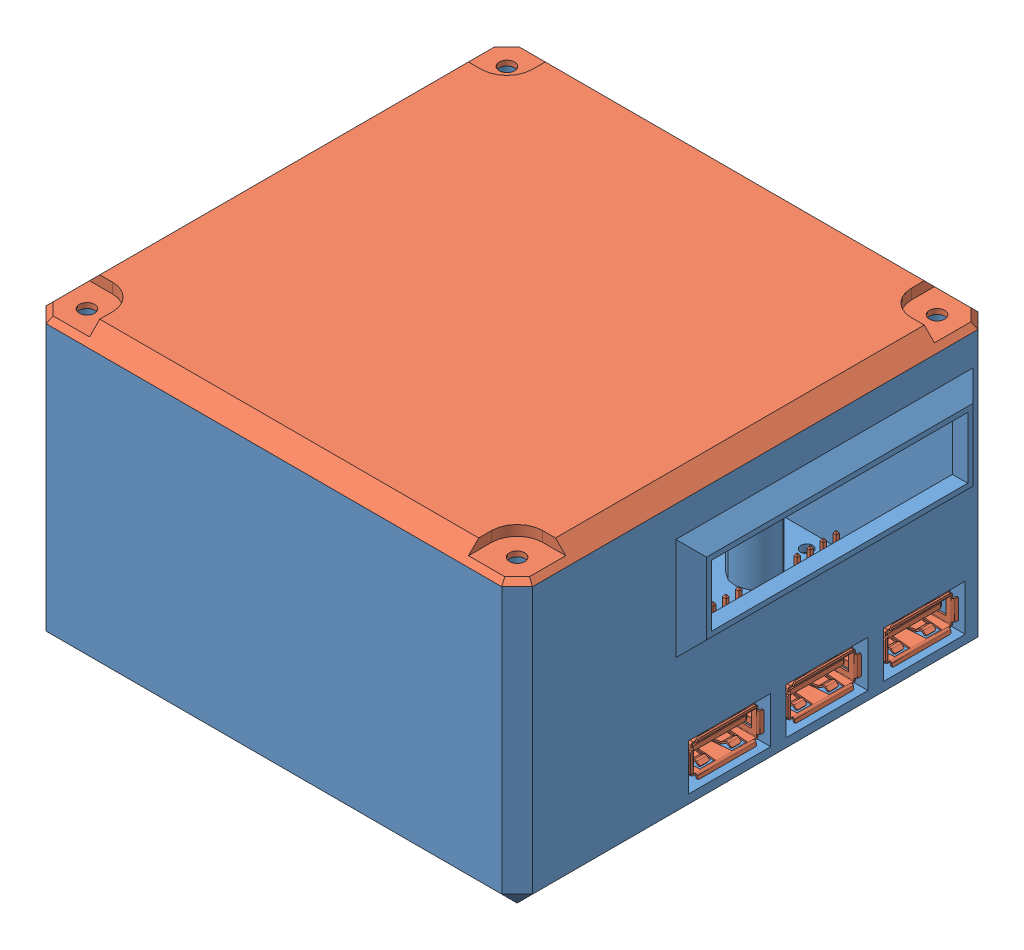
SolidWorks assembly NEW Arduino Case Assembly, configuration Default. Lengths in mm.
Overall size (98 58 93).
56 component instances, 22 part files, 33 mates.
Components (placement in the parent):
- NEW Mega 2560 Pro embed Case-1: NEW Mega 2560 Pro embed Case [Default] at origin size (98 55 93)
- NEW Mega 2560 Pro embed Case LID-1: NEW Mega 2560 Pro embed Case LID [Default] at (0 56 0) size (95 3 93)
- MEGA 2560 PRO (EMBED)-1: MEGA 2560 PRO (EMBED) [Default] at (-24.5 4 -15.5) x (1 0 0) z (0 1 0) size (38 54.09 6.02)
  - MEGA 2560 PRO (EMBED)(2)^MEGA 2560 PRO (EMBED)-1: MEGA 2560 PRO (EMBED)(2)^MEGA 2560 PRO (EMBED) [Default] at origin size (38 54.09 6.02) (virtual)
    - Mega 2560 Pro - Board^MEGA 2560 PRO (EMBED)(2)_MEGA 2560 PRO (EMBED)-1: Mega 2560 Pro - Board^MEGA 2560 PRO (EMBED)(2)_MEGA 2560 PRO (EMBED) [Default] at origin size (38 54 1.78) (virtual)
    - SOT223-3^MEGA 2560 PRO (EMBED)(2)_MEGA 2560 PRO (EMBED)-1: SOT223-3^MEGA 2560 PRO (EMBED)(2)_MEGA 2560 PRO (EMBED) [Default] at (-7.7036 13.3224 1.6256) x (-1 0 0) z (0 0 1) size (6.5 7.07 1.6) (virtual)
    - SOT223-3^MEGA 2560 PRO (EMBED)(2)_MEGA 2560 PRO (EMBED)-2: SOT223-3^MEGA 2560 PRO (EMBED)(2)_MEGA 2560 PRO (EMBED) [Default] at (-7.5781 23.9617 1.6256) x (-1 0 0) z (0 0 1) size (6.5 7.07 1.6) (virtual)
    - ATmega2560-16AU^MEGA 2560 PRO (EMBED)(2)_MEGA 2560 PRO (EMBED)-1: ATmega2560-16AU^MEGA 2560 PRO (EMBED)(2)_MEGA 2560 PRO (EMBED) [Default] at (0.2253 -9.3836 1.5256) x (0.707107 -0.707107 0) z (0 0 1) size (16 16 1.21) (virtual)
    - SOIC -16^MEGA 2560 PRO (EMBED)(2)_MEGA 2560 PRO (EMBED)-1: SOIC -16^MEGA 2560 PRO (EMBED)(2)_MEGA 2560 PRO (EMBED) [Default] at (0.546 8.9647 1.4756) x (0 1 0) z (1 0 0) size (6 1.4 9.9) (virtual)
    - Crystal Oscillator (SMD)^MEGA 2560 PRO (EMBED)(2)_MEGA 2560 PRO (EMBED)-1: Crystal Oscillator (SMD)^MEGA 2560 PRO (EMBED)(2)_MEGA 2560 PRO (EMBED) [Default] at (-10.7852 -19.6364 2.54) x (0 -1 0) z (0 0 1) size (13.06 4.55 4.32) (virtual)
    - Crystal Oscillator (SMD)^MEGA 2560 PRO (EMBED)(2)_MEGA 2560 PRO (EMBED)-2: Crystal Oscillator (SMD)^MEGA 2560 PRO (EMBED)(2)_MEGA 2560 PRO (EMBED) [Default] at (10.6809 3.6875 2.54) x (0 -1 0) z (0 0 1) size (13.06 4.55 4.32) (virtual)
    - 1206 Capacitor^MEGA 2560 PRO (EMBED)(2)_MEGA 2560 PRO (EMBED)-1: 1206 Capacitor^MEGA 2560 PRO (EMBED)(2)_MEGA 2560 PRO (EMBED) [Default] at (-3.8106 17.9279 1.6231) x (0 -1 0) z (0 0 1) size (3.2 1.6 1.6) (virtual)
    - Fuse (1206) - Green^MEGA 2560 PRO (EMBED)(2)_MEGA 2560 PRO (EMBED)-1: Fuse (1206) - Green^MEGA 2560 PRO (EMBED)(2)_MEGA 2560 PRO (EMBED) [Default] at (-0.2207 16.3875 1.6281) x (0 -1 0) z (0 0 1) size (3.28 1.75 0.87) (virtual)
    - Diode - SMD - DO-214AC^MEGA 2560 PRO (EMBED)(2)_MEGA 2560 PRO (EMBED)-1: Diode - SMD - DO-214AC^MEGA 2560 PRO (EMBED)(2)_MEGA 2560 PRO (EMBED) [Default] at (-1.7706 25.543 1.4756) x (0 -1 0) z (0 0 1) size (5.6 2.95 2.91) (virtual)
    - USB - Micro^MEGA 2560 PRO (EMBED)(2)_MEGA 2560 PRO (EMBED)-1: USB - Micro^MEGA 2560 PRO (EMBED)(2)_MEGA 2560 PRO (EMBED) [Default] at (2.2104 21.1734 1.3475) x (-1 0 0) z (0 1 0) size (7.92 3.01 5.67) (virtual)
    - 0603 Capacitor^MEGA 2560 PRO (EMBED)(2)_MEGA 2560 PRO (EMBED)-1: 0603 Capacitor^MEGA 2560 PRO (EMBED)(2)_MEGA 2560 PRO (EMBED) [Default] at (10.7145 18.9901 1.6231) x (0 -1 0) z (0 0 1) size (1.6 0.84 0.84) (virtual)
    - 0603 Capacitor^MEGA 2560 PRO (EMBED)(2)_MEGA 2560 PRO (EMBED)-2: 0603 Capacitor^MEGA 2560 PRO (EMBED)(2)_MEGA 2560 PRO (EMBED) [Default] at (4.611 3.4374 1.6231) x (0 -1 0) z (0 0 1) size (1.6 0.84 0.84) (virtual)
    - 0603 Capacitor^MEGA 2560 PRO (EMBED)(2)_MEGA 2560 PRO (EMBED)-3: 0603 Capacitor^MEGA 2560 PRO (EMBED)(2)_MEGA 2560 PRO (EMBED) [Default] at (7.1573 7.8647 1.6231) x (0 1 0) z (0 0 1) size (1.6 0.84 0.84) (virtual)
    - 0603 Capacitor^MEGA 2560 PRO (EMBED)(2)_MEGA 2560 PRO (EMBED)-4: 0603 Capacitor^MEGA 2560 PRO (EMBED)(2)_MEGA 2560 PRO (EMBED) [Default] at (7.0977 13.4599 1.6231) x (0 1 0) z (0 0 1) size (1.6 0.84 0.84) (virtual)
    - 0603 Capacitor^MEGA 2560 PRO (EMBED)(2)_MEGA 2560 PRO (EMBED)-5: 0603 Capacitor^MEGA 2560 PRO (EMBED)(2)_MEGA 2560 PRO (EMBED) [Default] at (5.1576 -19.4722 1.6231) x (0 1 0) z (1 0 0) size (1.6 0.84 0.84) (virtual)
    - 0603 Capacitor^MEGA 2560 PRO (EMBED)(2)_MEGA 2560 PRO (EMBED)-6: 0603 Capacitor^MEGA 2560 PRO (EMBED)(2)_MEGA 2560 PRO (EMBED) [Default] at (-10.8858 1.8771 1.6231) x (0 1 0) z (1 0 0) size (1.6 0.84 0.84) (virtual)
    - 0603 Capacitor^MEGA 2560 PRO (EMBED)(2)_MEGA 2560 PRO (EMBED)-7: 0603 Capacitor^MEGA 2560 PRO (EMBED)(2)_MEGA 2560 PRO (EMBED) [Default] at (2.9599 3.4697 1.6231) x (0 -1 0) z (0 0 1) size (1.6 0.84 0.84) (virtual)
    - 0603 Capacitor^MEGA 2560 PRO (EMBED)(2)_MEGA 2560 PRO (EMBED)-8: 0603 Capacitor^MEGA 2560 PRO (EMBED)(2)_MEGA 2560 PRO (EMBED) [Default] at (2.0157 3.7447 1.6231) x (-1 0 0) z (0 0 1) size (1.6 0.84 0.84) (virtual)
    - 0603 Capacitor^MEGA 2560 PRO (EMBED)(2)_MEGA 2560 PRO (EMBED)-9: 0603 Capacitor^MEGA 2560 PRO (EMBED)(2)_MEGA 2560 PRO (EMBED) [Default] at (-8.0885 -1.9063 1.6231) x (0 1 0) z (1 0 0) size (1.6 0.84 0.84) (virtual)
    - 0603 Capacitor^MEGA 2560 PRO (EMBED)(2)_MEGA 2560 PRO (EMBED)-10: 0603 Capacitor^MEGA 2560 PRO (EMBED)(2)_MEGA 2560 PRO (EMBED) [Default] at (-3.7884 20.5934 1.6231) x (0 1 0) z (0 0 1) size (1.6 0.84 0.84) (virtual)
    - 0603 Capacitor^MEGA 2560 PRO (EMBED)(2)_MEGA 2560 PRO (EMBED)-11: 0603 Capacitor^MEGA 2560 PRO (EMBED)(2)_MEGA 2560 PRO (EMBED) [Default] at (-8.8216 3.4762 1.6231) x (0 -1 0) z (0 0 1) size (1.6 0.84 0.84) (virtual)
    - 0603 Capacitor^MEGA 2560 PRO (EMBED)(2)_MEGA 2560 PRO (EMBED)-12: 0603 Capacitor^MEGA 2560 PRO (EMBED)(2)_MEGA 2560 PRO (EMBED) [Default] at (6.3032 3.4697 2.4613) x (0 -1 0) z (1 0 0) size (1.6 0.84 0.84) (virtual)
    - 0603 Capacitor^MEGA 2560 PRO (EMBED)(2)_MEGA 2560 PRO (EMBED)-13: 0603 Capacitor^MEGA 2560 PRO (EMBED)(2)_MEGA 2560 PRO (EMBED) [Default] at (-6.2819 -20.9115 1.6231) x (-1 0 0) z (0 1 0) size (1.6 0.84 0.84) (virtual)
    - 0603 Capacitor^MEGA 2560 PRO (EMBED)(2)_MEGA 2560 PRO (EMBED)-14: 0603 Capacitor^MEGA 2560 PRO (EMBED)(2)_MEGA 2560 PRO (EMBED) [Default] at (-7.8888 -17.889 1.6231) size (1.6 0.84 0.84) (virtual)
    - 0603 Resistor^MEGA 2560 PRO (EMBED)(2)_MEGA 2560 PRO (EMBED)-1: 0603 Resistor^MEGA 2560 PRO (EMBED)(2)_MEGA 2560 PRO (EMBED) [Default] at (-6.1185 1.9325 1.6231) x (0 1 0) z (0 0 1) size (1.6 0.85 0.56) (virtual)
    - 0603 Resistor^MEGA 2560 PRO (EMBED)(2)_MEGA 2560 PRO (EMBED)-2: 0603 Resistor^MEGA 2560 PRO (EMBED)(2)_MEGA 2560 PRO (EMBED) [Default] at (-8.697 -1.8307 1.6231) x (0 1 0) z (0 0 1) size (1.6 0.85 0.56) (virtual)
    - 0603 Resistor^MEGA 2560 PRO (EMBED)(2)_MEGA 2560 PRO (EMBED)-3: 0603 Resistor^MEGA 2560 PRO (EMBED)(2)_MEGA 2560 PRO (EMBED) [Default] at (-10.3133 -1.7908 1.6231) x (0 1 0) z (0 0 1) size (1.6 0.85 0.56) (virtual)
    - 0603 Resistor^MEGA 2560 PRO (EMBED)(2)_MEGA 2560 PRO (EMBED)-4: 0603 Resistor^MEGA 2560 PRO (EMBED)(2)_MEGA 2560 PRO (EMBED) [Default] at (6.8981 17.2332 1.6231) x (0 1 0) z (0 0 1) size (1.6 0.85 0.56) (virtual)
    - 0603 Resistor^MEGA 2560 PRO (EMBED)(2)_MEGA 2560 PRO (EMBED)-5: 0603 Resistor^MEGA 2560 PRO (EMBED)(2)_MEGA 2560 PRO (EMBED) [Default] at (-4.1536 1.9449 1.6231) x (0 1 0) z (0 0 1) size (1.6 0.85 0.56) (virtual)
    - 0603 Resistor^MEGA 2560 PRO (EMBED)(2)_MEGA 2560 PRO (EMBED)-6: 0603 Resistor^MEGA 2560 PRO (EMBED)(2)_MEGA 2560 PRO (EMBED) [Default] at (7.1292 10.6782 1.6231) x (0 1 0) z (0 0 1) size (1.6 0.85 0.56) (virtual)
    - 0603 Resistor^MEGA 2560 PRO (EMBED)(2)_MEGA 2560 PRO (EMBED)-7: 0603 Resistor^MEGA 2560 PRO (EMBED)(2)_MEGA 2560 PRO (EMBED) [Default] at (5.2754 17.2903 1.6231) x (0 1 0) z (0 0 1) size (1.6 0.85 0.56) (virtual)
    - 0603 Resistor^MEGA 2560 PRO (EMBED)(2)_MEGA 2560 PRO (EMBED)-8: 0603 Resistor^MEGA 2560 PRO (EMBED)(2)_MEGA 2560 PRO (EMBED) [Default] at (9.8818 17.3443 1.6231) x (0 1 0) z (0 0 1) size (1.6 0.85 0.56) (virtual)
    - 0603 Resistor^MEGA 2560 PRO (EMBED)(2)_MEGA 2560 PRO (EMBED)-9: 0603 Resistor^MEGA 2560 PRO (EMBED)(2)_MEGA 2560 PRO (EMBED) [Default] at (-11.9263 1.9088 1.6231) x (0 1 0) z (0 0 1) size (1.6 0.85 0.56) (virtual)
    - 0603 Resistor^MEGA 2560 PRO (EMBED)(2)_MEGA 2560 PRO (EMBED)-10: 0603 Resistor^MEGA 2560 PRO (EMBED)(2)_MEGA 2560 PRO (EMBED) [Default] at (7.18 4.9009 1.6231) x (0 1 0) z (0 0 1) size (1.6 0.85 0.56) (virtual)
    - 0603 Resistor^MEGA 2560 PRO (EMBED)(2)_MEGA 2560 PRO (EMBED)-11: 0603 Resistor^MEGA 2560 PRO (EMBED)(2)_MEGA 2560 PRO (EMBED) [Default] at (-11.9146 -1.6797 1.6231) x (0 1 0) z (0 0 1) size (1.6 0.85 0.56) (virtual)
    - 0603 Resistor^MEGA 2560 PRO (EMBED)(2)_MEGA 2560 PRO (EMBED)-12: 0603 Resistor^MEGA 2560 PRO (EMBED)(2)_MEGA 2560 PRO (EMBED) [Default] at (-6.3495 -18.5603 1.6231) x (-1 0 0) z (0 0 1) size (1.6 0.85 0.56) (virtual)
    - LED - 0603 - Blue^MEGA 2560 PRO (EMBED)(2)_MEGA 2560 PRO (EMBED)-1: LED - 0603 - Blue^MEGA 2560 PRO (EMBED)(2)_MEGA 2560 PRO (EMBED) [Default] at (7.1908 -19.2239 1.6256) x (0 1 0) z (0 0 1) size (1.63 0.73 0.83) (virtual)
    - LED_-_Vishay_-_6063_-_Green^MEGA 2560 PRO (EMBED)(2)_MEGA 2560 PRO (EMBED)-1: LED_-_Vishay_-_6063_-_Green^MEGA 2560 PRO (EMBED)(2)_MEGA 2560 PRO (EMBED) [Default] at (10.6783 -18.0475 1.5956) x (0 -1 0) z (0 0 1) size (1.63 0.73 0.83) (virtual)
    - LED - 0603 - Blue^MEGA 2560 PRO (EMBED)(2)_MEGA 2560 PRO (EMBED)-2: LED - 0603 - Blue^MEGA 2560 PRO (EMBED)(2)_MEGA 2560 PRO (EMBED) [Default] at (9.0246 -17.9783 1.6256) x (0 -1 0) z (0 0 1) size (1.63 0.73 0.83) (virtual)
    - 1206 Fuse^MEGA 2560 PRO (EMBED)(2)_MEGA 2560 PRO (EMBED)-1: 1206 Fuse^MEGA 2560 PRO (EMBED)(2)_MEGA 2560 PRO (EMBED) [Default] at (1.6964 17.9461 1.6231) x (0 -1 0) z (0 0 1) size (3.2 1.6 0.53) (virtual)
    - SWT-32^MEGA 2560 PRO (EMBED)(2)_MEGA 2560 PRO (EMBED)-1: SWT-32^MEGA 2560 PRO (EMBED)(2)_MEGA 2560 PRO (EMBED) [Default] at (15.7781 21.6695 1.6256) x (0 1 0) z (0 0 1) size (8 6.4 2.9) (virtual)
    - LED - 0603 - Blue^MEGA 2560 PRO (EMBED)(2)_MEGA 2560 PRO (EMBED)-3: LED - 0603 - Blue^MEGA 2560 PRO (EMBED)(2)_MEGA 2560 PRO (EMBED) [Default] at (12.5463 -18.1103 1.6256) x (0 -1 0) z (0 0 1) size (1.63 0.73 0.83) (virtual)
- PCB2x8-1: PCB2x8 [Default] at (-40 4 22.45) x (0 0 1) z (-1 0 0) size (20.05 1.23 80.2)
- Servo Driver-1: Servo Driver [Default] at (8.825 4 -11.4) x (0 0 1) z (-1 0 0) size (62.2 14.3 25.35)
- USB Type A Female Breakout-1: USB Type A Female Breakout [Default] at (41.5 4 -33) x (0 0 -1) z (0 1 0) size (17 22.55 12.12)
- USB Type A Female Breakout-2: USB Type A Female Breakout [Default] at (41.5 4 -14) x (0 0 -1) z (0 1 0) size (17 22.55 12.12)
- USB Type A Female Breakout-3: USB Type A Female Breakout [Default] at (41.5 4 5) x (0 0 -1) z (0 1 0) size (17 22.55 12.12)
- Upper PCB harness-1: Upper PCB harness [Default] at (40.2 34.125 40) x (0 0 -1) z (1 0 0) size (65.5 3.5 88)
  - PCB2x8-1: PCB2x8 [Default] at origin size (20.05 1.23 80.2)
  - PCB harness-1: PCB harness [Default] at (10 -1.5 -40.2) x (0 0 -1) z (1 0 0) size (88 3.5 65.5)
- Moveo Logo light-1: Moveo Logo light [Default] at (6.05 34.125 -1.5) x (0 0 -1) z (1 0 0) size (40 10.14 20)
Mates (geometry in assembly coordinates):
- Coincident1: coordinate: point of NEW Mega 2560 Pro embed Case-1
- Coincident2: coincident aligned: plane of NEW Mega 2560 Pro embed Case-1 through (0 0 0) normal (0 0 1); plane of NEW Mega 2560 Pro embed Case LID-1 through (0 56 0) normal (0 0 1)
- Coincident3: coincident aligned: plane of NEW Mega 2560 Pro embed Case-1 through (0 0 0) normal (1 0 0); plane of NEW Mega 2560 Pro embed Case LID-1 through (0 56 0) normal (1 0 0)
- Coincident4: coincident anti-aligned: plane of NEW Mega 2560 Pro embed Case-1 through (0 55 0) normal (0 1 0); plane of NEW Mega 2560 Pro embed Case LID-1 through (0 55 0) normal (0 -1 0)
- Parallel1: parallel anti-aligned: plane of NEW Mega 2560 Pro embed Case-1 through (0 55 43.5) normal (0 0 -1); plane of PCB2x8-1 through (-40 4 42.5) normal (0 0 1)
- Distance1: distance = 2 mm anti-aligned: plane of PCB2x8-1 through (0.1 4 32.475) normal (0 -1 0); plane of NEW Mega 2560 Pro embed Case-1 through (0 2 0) normal (0 1 0)
- Distance2: distance = 2 mm anti-aligned: plane of MEGA 2560 PRO (EMBED)-1/MEGA 2560 PRO (EMBED)(2)^MEGA 2560 PRO (EMBED)-1/Mega 2560 Pro - Board^MEGA 2560 PRO (EMBED)(2)_MEGA 2560 PRO (EMBED)-1 through (-24.5 4 -15.5) normal (0 -1 0); plane of NEW Mega 2560 Pro embed Case-1 through (0 2 0) normal (0 1 0)
- Distance3: distance = 1 mm anti-aligned: plane of MEGA 2560 PRO (EMBED)-1/MEGA 2560 PRO (EMBED)(2)^MEGA 2560 PRO (EMBED)-1/Mega 2560 Pro - Board^MEGA 2560 PRO (EMBED)(2)_MEGA 2560 PRO (EMBED)-1 through (-43.5 5.6256 -42.5) normal (0 0 -1); plane of NEW Mega 2560 Pro embed Case-1 through (0 55 -43.5) normal (0 0 1)
- Distance4: distance = 1 mm anti-aligned: plane of MEGA 2560 PRO (EMBED)-1/MEGA 2560 PRO (EMBED)(2)^MEGA 2560 PRO (EMBED)-1/Mega 2560 Pro - Board^MEGA 2560 PRO (EMBED)(2)_MEGA 2560 PRO (EMBED)-1 through (-43.5 5.6256 11.5) normal (-1 0 0); plane of NEW Mega 2560 Pro embed Case-1 through (-44.5 55 0) normal (1 0 0)
- Coincident10: coincident aligned: plane of PCB2x8-1 through (-40 4 22.45) normal (-1 0 0); plane of PCB2x8-2 through (-42.5 30.21 20.7) normal (-1 0 0)
- Distance5: distance = 25 mm anti-aligned: plane of PCB2x8-2 through (-2.4 30.21 30.725) normal (0 -1 0); plane of PCB2x8-1 through (0.1 5.21 32.475) normal (0 1 0)
- Coincident12: coincident aligned: plane of PCB2x8-1 through (40.2 4 22.45) normal (0 0 -1); plane of PCB2x8-2 through (37.7 30.21 20.7) normal (0 0 -1)
- Distance7: distance = 1 mm anti-aligned: plane of Servo Driver-1 through (-2.85 5.4 -42.5) normal (0 0 -1); plane of NEW Mega 2560 Pro embed Case-1 through (0 55 -43.5) normal (0 0 1)
- Distance8: distance = 2 mm anti-aligned: plane of Servo Driver-1 through (-2.85 4 -41.5) normal (0 -1 0); plane of NEW Mega 2560 Pro embed Case-1 through (0 2 0) normal (0 1 0)
- Distance9: distance = 3 mm anti-aligned: plane of USB Type A Female Breakout-1 through (41.5 4 -24.5) normal (1 0 0); plane of NEW Mega 2560 Pro embed Case-1 through (44.5 55 0) normal (-1 0 0)
- Distance10: distance = 2 mm anti-aligned: plane of USB Type A Female Breakout-1 through (33 4 -33) normal (0 -1 0); plane of NEW Mega 2560 Pro embed Case-1 through (0 2 0) normal (0 1 0)
- Distance11: distance = 2 mm anti-aligned: plane of NEW Mega 2560 Pro embed Case-1 through (0 55 -43.5) normal (0 0 1); plane of USB Type A Female Breakout-1 through (41.5 4 -41.5) normal (0 0 -1)
- Coincident20: coincident aligned: plane of USB Type A Female Breakout-1 through (33 5.2 -33) normal (0 1 0); plane of USB Type A Female Breakout-2 through (33 5.2 -14) normal (0 1 0)
- Coincident21: coincident aligned: plane of USB Type A Female Breakout-1 through (24.5 4 -41.5) normal (-1 0 0); plane of USB Type A Female Breakout-2 through (24.5 4 -22.5) normal (-1 0 0)
- Distance12: distance = 2 mm anti-aligned: plane of USB Type A Female Breakout-2 through (41.5 4 -22.5) normal (0 0 -1); plane of USB Type A Female Breakout-1 through (24.5 4 -24.5) normal (0 0 1)
- Coincident23: coincident aligned: plane of USB Type A Female Breakout-1 through (33 5.2 -33) normal (0 1 0); plane of USB Type A Female Breakout-3 through (33 5.2 5) normal (0 1 0)
- Coincident24: coincident aligned: plane of USB Type A Female Breakout-1 through (24.5 4 -41.5) normal (-1 0 0); plane of USB Type A Female Breakout-3 through (24.5 4 -3.5) normal (-1 0 0)
- Distance13: distance = 2 mm anti-aligned: plane of USB Type A Female Breakout-2 through (24.5 4 -5.5) normal (0 0 1); plane of USB Type A Female Breakout-3 through (41.5 4 -3.5) normal (0 0 -1)
- Distance14: distance = 3 mm anti-aligned: plane of Servo Driver-1 through (21.5 5.4 -41.5) normal (1 0 0); plane of USB Type A Female Breakout-1 through (24.5 4 -41.5) normal (-1 0 0)
- Distance15: distance = 1 mm anti-aligned: plane of PCB2x8-1 through (-40 4 42.5) normal (0 0 1); plane of NEW Mega 2560 Pro embed Case-1 through (0 55 43.5) normal (0 0 -1)
- Coincident25: coincident aligned: plane of PCB2x8-1 through (-40 4 22.45) normal (-1 0 0); plane of Upper PCB harness-1/PCB2x8-1 through (-40 34.125 19.95) normal (-1 0 0)
- Distance16: distance = 25 mm anti-aligned: plane of Upper PCB harness-1/PCB harness-1 through (0 32.625 30) normal (0 -1 0); plane of PCB2x8-1 through (0.1 5.21 32.475) normal (0 1 0)
- Coincident28: coincident anti-aligned: plane of Upper PCB harness-1/PCB harness-1 through (0 32.625 30) normal (-1 0 0)
- Coincident29: coincident anti-aligned: plane of NEW Mega 2560 Pro embed Case-1 through (44.5 35 19.5) normal (0 -1 0); plane of Upper PCB harness-1/PCB harness-1 through (44 35 18) normal (0 1 0)
- Parallel2: parallel anti-aligned: plane of NEW Mega 2560 Pro embed Case-1 through (0 55 -43.5) normal (0 0 1); plane of Moveo Logo light-1 through (16.05 35.565 -21.5) normal (0 0 -1)
- Coincident30: coincident anti-aligned: plane of Upper PCB harness-1/PCB harness-1 through (0 34.125 30) normal (0 1 0); plane of Moveo Logo light-1 through (6.05 34.125 -1.5) normal (0 -1 0)
- Concentric1: concentric aligned: cylinder of Upper PCB harness-1/PCB harness-1 through (14 32.625 -19.45) axis (0 1 0) radius 1; cylinder of Moveo Logo light-1 through (14 34.125 -19.45) axis (0 1 0) radius 1
- Distance17: distance = 1.5 mm anti-aligned: plane of Upper PCB harness-1/PCB harness-1 through (42 34.125 42) normal (0 0 1); plane of NEW Mega 2560 Pro embed Case-1 through (0 55 43.5) normal (0 0 -1)
